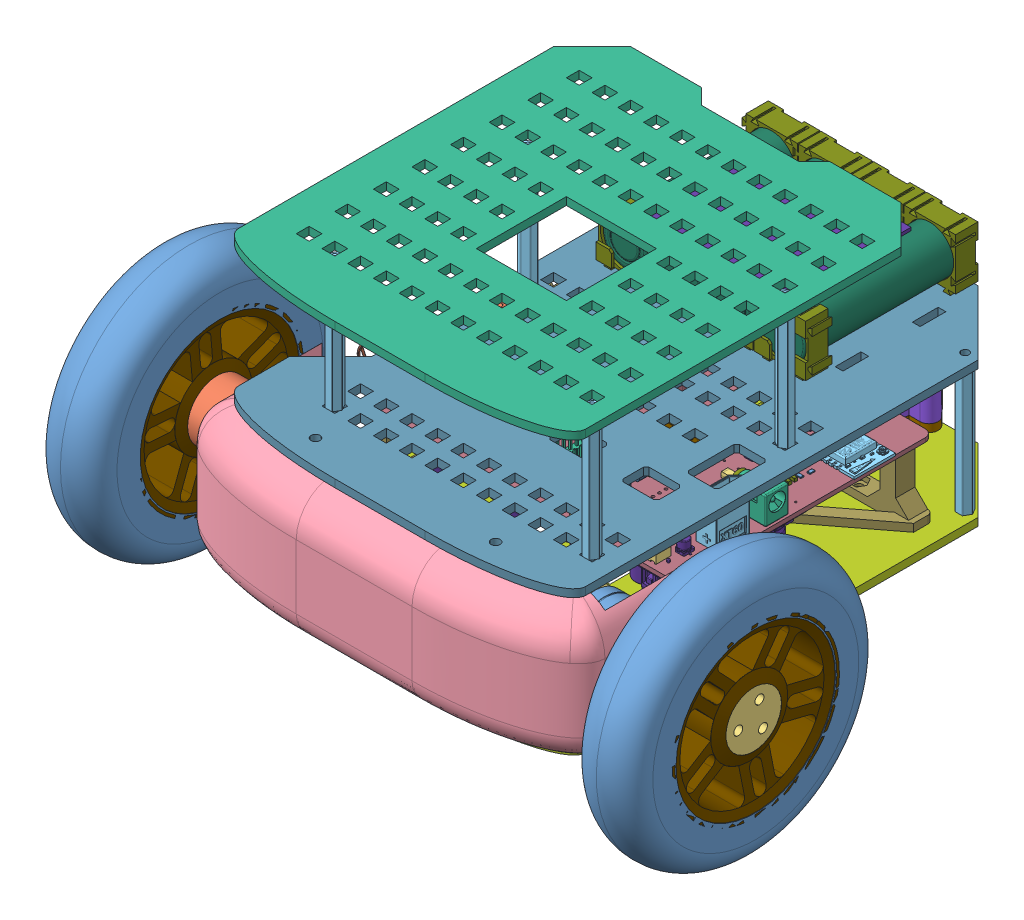
SolidWorks assembly main_assembly, configuration Predeterminado. Lengths in mm.
Overall size (232.39 147.84 245.63).
315 component instances, 64 part files, 45 mates.
Components (placement in the parent):
- JA25-371-12V-1: JA25-371-12V [Predeterminado] at (-23.0941 198.6621 54.477) x (0 0 1) z (-1 0 0) size (25 25 76.39)
  - Gearbox-1: Gearbox [Predeterminado] at (16.9623 5.2379 20.5646) size (25 25 21)
  - hub-1: hub [Predeterminado] at (16.9623 5.2379 39.5646) x (0.985611 -0.169031 0) z (0 0 1) size (6.95 6.95 4.5)
  - Motor-1: Motor [Predeterminado] at (16.9623 5.2379 -9.9354) size (24.2 24.2 30.5)
  - Axis-1: Axis [Predeterminado] at (16.9623 5.2379 39.5646) x (0.853161 0.521648 0) z (0 0 1) size (4 4 14)
  - PCB-1: PCB [Predeterminado] at (16.9623 5.2379 -11.4354) x (-1 0 0) z (0 0 -1) size (23 23 4.73)
  - Magnet-1: Magnet [Predeterminado] at (16.9623 5.2379 -17.3254) x (-0.17817 -0.984 0) z (0 0 -1) size (14.2 14.2 15.5)
- JA25-371-12V-2: JA25-371-12V [Predeterminado] at (42.7766 209.1379 54.477) x (0 0 1) z (1 0 0) size (25 25 76.39)
  - Gearbox-1: Gearbox [Predeterminado] at (16.9623 5.2379 20.5646) size (25 25 21)
  - hub-1: hub [Predeterminado] at (16.9623 5.2379 39.5646) x (0.985611 -0.169031 0) z (0 0 1) size (6.95 6.95 4.5)
  - Motor-1: Motor [Predeterminado] at (16.9623 5.2379 -9.9354) size (24.2 24.2 30.5)
  - Axis-1: Axis [Predeterminado] at (16.9623 5.2379 39.5646) x (0.853161 0.521648 0) z (0 0 1) size (4 4 14)
  - PCB-1: PCB [Predeterminado] at (16.9623 5.2379 -11.4354) x (-1 0 0) z (0 0 -1) size (23 23 4.73)
  - Magnet-1: Magnet [Predeterminado] at (16.9623 5.2379 -17.3254) x (-0.17817 -0.984 0) z (0 0 -1) size (14.2 14.2 15.5)
- base_noah-1: base_noah [Predeterminado] at (9.8412 177.5 6.4393) size (135.31 3.5 190.25)
- CasterJoint-1: CasterJoint [Default] at (-10.4939 224.3692 -36.408) x (1 0 0) z (0 0 -1) size (61 48.46 48.78)
  - C000-1: C000 [Default] at (20.3352 23.8692 48.4027) size (61 17 46)
  - C001-1: C001 [Default] at (20.3352 23.8692 48.4027) size (61 16.32 46)
  - BALL6MM-1: BALL6MM [Predeterminado] at (22.8352 26.8692 52.7329) size (6 6 6)
  - BALL40MM-1: BALL40MM [Default] at (20.3352 49.3191 48.4027) x (0.992761 -0.035378 0.11478) z (-0.109645 0.123176 0.986309) size (40 40 40)
  - BALL6MM-2: BALL6MM [Predeterminado] at (22.8352 26.8692 44.0726) size (6 6 6)
  - BALL6MM-3: BALL6MM [Predeterminado] at (15.3352 26.8692 48.4027) size (6 6 6)
  - pan head cross collar screw_din-1: pan head cross collar screw_din [DIN 967 - M3 x 10 - Z --- 9C] at (-6.6648 46.2192 48.6527) x (0 -1 0) z (0.01313 0 0.999914) size (12.25 7.5 7.5) (hidden)
  - pan head cross collar screw_din-2: pan head cross collar screw_din [DIN 967 - M3 x 10 - Z --- 9C] at (47.3352 46.2192 48.6527) x (0 -1 0) z (0 0 1) size (12.25 7.5 7.5) (hidden)
- pcb_holder_noah-1: pcb_holder_noah [Default] at (-2.6116 180.5 18.9157) x (-1 0 0) z (0 0 -1) size (120 28 100)
- power_button_noah-1: power_button_noah [Default] at (-42.6588 193.5 -36.0607) x (0 0 1) z (-1 0 0) size (25 20 7.5)
- noah_v02-1: noah_v02 [Default] at (159.8412 208.5 96.4393) x (-1 0 0) z (0 1 0) size (125.96 104.91 49.76)
  - noah_v02.step-1: noah_v02.step [Default] at origin size (125.96 104.91 49.76)
    - IDC-Header_2x05_P2.54mm_Vertical.step-1: IDC-Header_2x05_P2.54mm_Vertical.step [Default] at (176.6 -132.6 1.65) x (-0.707107 0.707107 0) z (0 0 1) size (9.1 20.36 12.1)
      - SOLID.step-1: SOLID.step [Default] at origin size (9.1 20.36 12.1)
    - DFN-8-1EP_3x3mm_P0.5mm_EP1.66x2.38mm.step-1: DFN-8-1EP_3x3mm_P0.5mm_EP1.66x2.38mm.step [Default] at (105.305 -107.385 1.65) x (0 1 0) z (0 0 1) size (3 2.98 0.77)
      - SOLID-0.step-1: SOLID-0.step [Default] at origin size (3 2.98 0.77)
    - C_0805_2012Metric.step-1: C_0805_2012Metric.step [Default] at (160.4 -70.1 1.65) x (0 -1 0) z (0 0 1) size (2 1.25 1.25)
      - SOLID-1.step-1: SOLID-1.step [Default] at origin size (2 1.25 1.25)
    - CP_Elec_4x4.5.step-1: CP_Elec_4x4.5.step [Default] at (140.6 -65.3 1.65) x (0 -1 0) z (0 0 1) size (5.74 5.46 4.5)
      - SOLID-2.step-1: SOLID-2.step [Default] at origin size (5.74 5.46 4.5)
    - C_0805_2012Metric.step-2: C_0805_2012Metric.step [Default] at (115.6 -134.6 1.65) size (2 1.25 1.25)
      - SOLID-1.step-1: SOLID-1.step [Default] at origin size (2 1.25 1.25)
    - CP_Elec_4x4.5.step-2: CP_Elec_4x4.5.step [Default] at (114.6 -129.4 1.65) x (0 1 0) z (0 0 1) size (5.74 5.46 4.5)
      - SOLID-2.step-1: SOLID-2.step [Default] at origin size (5.74 5.46 4.5)
    - PinSocket_1x06_P2.54mm_Vertical.step-1: PinSocket_1x06_P2.54mm_Vertical.step [Default] at (153.2 -146.2 1.65) x (0 -1 0) z (0 0 1) size (2.54 15.24 10.1)
      - SOLID-3.step-1: SOLID-3.step [Default] at origin size (2.54 15.24 10.1)
    - PinSocket_2x06_P2.54mm_Vertical.step-1: PinSocket_2x06_P2.54mm_Vertical.step [Default] at (153.2 -142.6 1.65) x (0 -1 0) z (0 0 1) size (5.08 15.24 10.1)
      - SOLID-4.step-1: SOLID-4.step [Default] at origin size (5.08 15.24 10.1)
    - ublox_NEO-6M.step-1: ublox_NEO-6M.step [Default] at (181.8 -59.6 11.65) x (0 1 0) z (1 0 0) size (39.06 22.61 48.01)
      - COMPOUND.step-1: COMPOUND.step [Default] at origin size (39.06 22.61 48.01)
    - D_SMA.step-1: D_SMA.step [Default] at (198.4 -143.2 1.65) x (-1 0 0) z (0 0 1) size (5 2.7 2.22)
      - SOLID-5.step-1: SOLID-5.step [Default] at origin size (5 2.7 2.22)
    - PinHeader_1x03_P2.54mm_Vertical.step-1: PinHeader_1x03_P2.54mm_Vertical.step [Default] at (105.6 -147.4 1.65) x (-1 0 0) z (0 0 1) size (2.54 7.62 11.54)
      - SOLID-6.step-1: SOLID-6.step [Default] at origin size (2.54 7.62 11.54)
    - C_0805_2012Metric.step-3: C_0805_2012Metric.step [Default] at (101.3 -107.1 1.65) x (-1 0 0) z (0 0 1) size (2 1.25 1.25)
      - SOLID-1.step-1: SOLID-1.step [Default] at origin size (2 1.25 1.25)
    - C_0805_2012Metric.step-4: C_0805_2012Metric.step [Default] at (101.3 -104.8 1.65) x (-1 0 0) z (0 0 1) size (2 1.25 1.25)
      - SOLID-1.step-1: SOLID-1.step [Default] at origin size (2 1.25 1.25)
    - ESP07.step-1: ESP07.step [Default] at (101.6 -127.3 1.65) x (0 1 0) z (1 0 0) size (19.34 14.61 27.24)
      - COMPOUND-7.step-1: COMPOUND-7.step [Default] at origin size (19.34 14.61 27.24)
    - Power_Barrel_Connector_Jack_694106301002.step-1: Power_Barrel_Connector_Jack_694106301002.step [Default] at (104.13 -90.01 1.65) x (0 -1 0) z (0 0 1) size (9.49 14.48 14.52)
      - COMPOUND-8.step-1: COMPOUND-8.step [Default] at origin size (9.49 14.48 14.52)
    - GY-91.step-1: GY-91.step [Default] at (119 -134.7 9.65) size (14.4 21 11.75)
      - COMPOUND-9.step-1: COMPOUND-9.step [Default] at origin size (14.4 21 11.75)
    - Tact_Switch_4.5mm_SMT.step-1: Tact_Switch_4.5mm_SMT.step [Default] at (139.14 -127.61 1.65) x (0 1 0) z (0 0 1) size (7.5 4.5 4.2)
      - COMPOUND-10.step-1: COMPOUND-10.step [Default] at origin size (7.5 4.5 4.2)
    - Tact_Switch_4.5mm_SMT.step-2: Tact_Switch_4.5mm_SMT.step [Default] at (167.3 -90.93 1.65) x (0 -1 0) z (0 0 1) size (7.5 4.5 4.2)
      - COMPOUND-10.step-1: COMPOUND-10.step [Default] at origin size (7.5 4.5 4.2)
    - tb5p-2p_p5_l10_w7-6_h10.step-1: tb5p-2p_p5_l10_w7-6_h10.step [Default] at (205.55 -62.68 6.65) x (0 1 0) z (1 0 0) size (10.6 14.1 7.6)
      - COMPOUND-11.step-1: COMPOUND-11.step [Default] at origin size (10.6 14.1 7.6)
    - SW_DIP_SPSTx02_Slide_6.7x6.64mm_W7.62mm_P2.54mm_LowProfile.step-1: SW_DIP_SPSTx02_Slide_6.7x6.64mm_W7.62mm_P2.54mm_LowProfile.step [Default] at (131.45 -139.55 1.65) x (-1 0 0) z (0 0 1) size (6.64 7.82 6)
      - SOLID-12.step-1: SOLID-12.step [Default] at origin size (6.64 7.82 6)
    - LQFP-100_14x14mm_P0.5mm.step-1: LQFP-100_14x14mm_P0.5mm.step [Default] at (161.4 -120.1 1.65) x (0.707107 -0.707107 0) z (0 0 1) size (16 16 1.5)
      - SOLID-13.step-1: SOLID-13.step [Default] at origin size (16 16 1.5)
    - USB_Mini-B_Lumberg_2486_01_Horizontal.step-1: USB_Mini-B_Lumberg_2486_01_Horizontal.step [Default] at (203.6 -123.9 1.65) x (0 1 0) z (0 0 1) size (9.9 9.21 5)
      - SOLID-14.step-1: SOLID-14.step [Default] at origin size (9.9 9.21 5)
    - Crystal_HC49-U_Vertical.step-1: Crystal_HC49-U_Vertical.step [Default] at (151.7 -106.6 1.65) x (-0.707107 -0.707107 0) z (0 0 1) size (10.9 4.65 16)
      - SOLID-15.step-1: SOLID-15.step [Default] at origin size (10.9 4.65 16)
    - SOIC-8_3.9x4.9mm_P1.27mm.step-1: SOIC-8_3.9x4.9mm_P1.27mm.step [Default] at (190.4 -107.7 1.65) size (6 4.9 1.75)
      - SOLID-16.step-1: SOLID-16.step [Default] at origin size (6 4.9 1.75)
    - SOT-23-5.step-1: SOT-23-5.step [Default] at (201.6 -138 1.65) size (2.8 2.9 1.55)
      - SOLID-17.step-1: SOLID-17.step [Default] at origin size (2.8 2.9 1.55)
    - SOT-23-6.step-1: SOT-23-6.step [Default] at (193.5 -124.3 1.65) size (2.8 2.9 1.55)
      - SOLID-18.step-1: SOLID-18.step [Default] at origin size (2.8 2.9 1.55)
    - XL4015_StepDown_DC-DC_5A_(CC-CV)_v1.step-1: XL4015_StepDown_DC-DC_5A_(CC-CV)_v1.step [Default] at (119.3 -102.3 -0.05) x (0 1 0) z (0 0 -1) size (51 26 18.15)
      - COMPOUND-19.step-1: COMPOUND-19.step [Default] at origin size (51 26 18.15)
    - XL4015_StepDown_DC-DC_5A_(CC-CV)_v1.step-2: XL4015_StepDown_DC-DC_5A_(CC-CV)_v1.step [Default] at (147.1 -102.4 -0.05) x (0 1 0) z (0 0 -1) size (51 26 18.15)
      - COMPOUND-19.step-1: COMPOUND-19.step [Default] at origin size (51 26 18.15)
    - XL4015_StepDown_DC-DC_5A_(CC-CV)_v1.step-3: XL4015_StepDown_DC-DC_5A_(CC-CV)_v1.step [Default] at (174.9 -102.3 -0.05) x (0 1 0) z (0 0 -1) size (51 26 18.15)
      - COMPOUND-19.step-1: COMPOUND-19.step [Default] at origin size (51 26 18.15)
    - XL4015_StepDown_DC-DC_5A_(CC-CV)_v1.step-4: XL4015_StepDown_DC-DC_5A_(CC-CV)_v1.step [Default] at (91.5 -102.3 -0.05) x (0 1 0) z (0 0 -1) size (51 26 18.15)
      - COMPOUND-19.step-1: COMPOUND-19.step [Default] at origin size (51 26 18.15)
    - TB6612FNG_Motor_Driver.step-1: TB6612FNG_Motor_Driver.step [Default] at (130.68 -80.59 11.65) x (0 0 1) z (1 0 0) size (3.57 20.98 20.9)
      - SOLID-20.step-1: SOLID-20.step [Default] at origin size (3.57 20.98 20.9)
    - R_0805_2012Metric.step-1: R_0805_2012Metric.step [Default] at (168.4 -107.4 1.65) x (0.707107 -0.707107 0) z (0 0 1) size (2 1.2 0.45)
      - SOLID-21.step-1: SOLID-21.step [Default] at origin size (2 1.2 0.45)
    - R_0805_2012Metric.step-2: R_0805_2012Metric.step [Default] at (200.7 -105.4 1.65) x (0 1 0) z (0 0 1) size (2 1.2 0.45)
      - SOLID-21.step-1: SOLID-21.step [Default] at origin size (2 1.2 0.45)
    - R_0805_2012Metric.step-3: R_0805_2012Metric.step [Default] at (200.7 -109.4 1.65) x (0 -1 0) z (0 0 1) size (2 1.2 0.45)
      - SOLID-21.step-1: SOLID-21.step [Default] at origin size (2 1.2 0.45)
    - R_0805_2012Metric.step-4: R_0805_2012Metric.step [Default] at (197.3 -105.4 1.65) x (0 1 0) z (0 0 1) size (2 1.2 0.45)
      - SOLID-21.step-1: SOLID-21.step [Default] at origin size (2 1.2 0.45)
    - R_0805_2012Metric.step-5: R_0805_2012Metric.step [Default] at (197.3 -109.4 1.65) x (0 -1 0) z (0 0 1) size (2 1.2 0.45)
      - SOLID-21.step-1: SOLID-21.step [Default] at origin size (2 1.2 0.45)
    - R_0805_2012Metric.step-6: R_0805_2012Metric.step [Default] at (192.1 -103.5 1.65) size (2 1.2 0.45)
      - SOLID-21.step-1: SOLID-21.step [Default] at origin size (2 1.2 0.45)
    - R_0805_2012Metric.step-7: R_0805_2012Metric.step [Default] at (201.6 -131.9 1.65) x (-1 0 0) z (0 0 1) size (2 1.2 0.45)
      - SOLID-21.step-1: SOLID-21.step [Default] at origin size (2 1.2 0.45)
    - R_0805_2012Metric.step-8: R_0805_2012Metric.step [Default] at (193.5 -120.9 1.65) size (2 1.2 0.45)
      - SOLID-21.step-1: SOLID-21.step [Default] at origin size (2 1.2 0.45)
    - R_0805_2012Metric.step-9: R_0805_2012Metric.step [Default] at (192.9 -127.5 1.65) x (-1 0 0) z (0 0 1) size (2 1.2 0.45)
      - SOLID-21.step-1: SOLID-21.step [Default] at origin size (2 1.2 0.45)
    - R_0805_2012Metric.step-10: R_0805_2012Metric.step [Default] at (192.9 -129.9 1.65) size (2 1.2 0.45)
      - SOLID-21.step-1: SOLID-21.step [Default] at origin size (2 1.2 0.45)
    - R_0805_2012Metric.step-11: R_0805_2012Metric.step [Default] at (110.6 -141.6 1.65) size (2 1.2 0.45)
      - SOLID-21.step-1: SOLID-21.step [Default] at origin size (2 1.2 0.45)
    - R_0805_2012Metric.step-12: R_0805_2012Metric.step [Default] at (177.2 -71.9 1.65) x (-1 0 0) z (0 0 1) size (2 1.2 0.45)
      - SOLID-21.step-1: SOLID-21.step [Default] at origin size (2 1.2 0.45)
    - R_0805_2012Metric.step-13: R_0805_2012Metric.step [Default] at (177.2 -65.3 1.65) x (-1 0 0) z (0 0 1) size (2 1.2 0.45)
      - SOLID-21.step-1: SOLID-21.step [Default] at origin size (2 1.2 0.45)
    - R_0805_2012Metric.step-14: R_0805_2012Metric.step [Default] at (177.2 -69.7 1.65) x (-1 0 0) z (0 0 1) size (2 1.2 0.45)
      - SOLID-21.step-1: SOLID-21.step [Default] at origin size (2 1.2 0.45)
    - R_0805_2012Metric.step-15: R_0805_2012Metric.step [Default] at (177.2 -67.5 1.65) x (-1 0 0) z (0 0 1) size (2 1.2 0.45)
      - SOLID-21.step-1: SOLID-21.step [Default] at origin size (2 1.2 0.45)
    - R_0805_2012Metric.step-16: R_0805_2012Metric.step [Default] at (165.3 -97.8 1.65) x (0 1 0) z (0 0 1) size (2 1.2 0.45)
      - SOLID-21.step-1: SOLID-21.step [Default] at origin size (2 1.2 0.45)
    - R_0805_2012Metric.step-17: R_0805_2012Metric.step [Default] at (152.4 -93.8 1.65) x (0 -1 0) z (0 0 1) size (2 1.2 0.45)
      - SOLID-21.step-1: SOLID-21.step [Default] at origin size (2 1.2 0.45)
    - R_0805_2012Metric.step-18: R_0805_2012Metric.step [Default] at (155.2 -93.8 1.65) x (0 -1 0) z (0 0 1) size (2 1.2 0.45)
      - SOLID-21.step-1: SOLID-21.step [Default] at origin size (2 1.2 0.45)
    - R_0805_2012Metric.step-19: R_0805_2012Metric.step [Default] at (192.9 -132.2 1.65) x (-1 0 0) z (0 0 1) size (2 1.2 0.45)
      - SOLID-21.step-1: SOLID-21.step [Default] at origin size (2 1.2 0.45)
    - R_0805_2012Metric.step-20: R_0805_2012Metric.step [Default] at (169 -104.8 1.65) x (0.707107 -0.707107 0) z (0 0 1) size (2 1.2 0.45)
      - SOLID-21.step-1: SOLID-21.step [Default] at origin size (2 1.2 0.45)
    - R_0805_2012Metric.step-21: R_0805_2012Metric.step [Default] at (174.7 -105.9 1.65) size (2 1.2 0.45)
      - SOLID-21.step-1: SOLID-21.step [Default] at origin size (2 1.2 0.45)
    - R_0805_2012Metric.step-22: R_0805_2012Metric.step [Default] at (111.4 -74.4 1.65) x (0 1 0) z (0 0 1) size (2 1.2 0.45)
      - SOLID-21.step-1: SOLID-21.step [Default] at origin size (2 1.2 0.45)
    - R_0805_2012Metric.step-23: R_0805_2012Metric.step [Default] at (110.4 -77.6 1.65) x (-1 0 0) z (0 0 1) size (2 1.2 0.45)
      - SOLID-21.step-1: SOLID-21.step [Default] at origin size (2 1.2 0.45)
    - R_0805_2012Metric.step-24: R_0805_2012Metric.step [Default] at (101.3 -109.5 1.65) size (2 1.2 0.45)
      - SOLID-21.step-1: SOLID-21.step [Default] at origin size (2 1.2 0.45)
    - R_0805_2012Metric.step-25: R_0805_2012Metric.step [Default] at (100.5 -113.1 1.65) x (0 -1 0) z (0 0 1) size (2 1.2 0.45)
      - SOLID-21.step-1: SOLID-21.step [Default] at origin size (2 1.2 0.45)
    - R_0805_2012Metric.step-26: R_0805_2012Metric.step [Default] at (115.4 -147.6 1.65) size (2 1.2 0.45)
      - SOLID-21.step-1: SOLID-21.step [Default] at origin size (2 1.2 0.45)
    - R_0805_2012Metric.step-27: R_0805_2012Metric.step [Default] at (115.4 -145.4 1.65) size (2 1.2 0.45)
      - SOLID-21.step-1: SOLID-21.step [Default] at origin size (2 1.2 0.45)
    - R_0805_2012Metric.step-28: R_0805_2012Metric.step [Default] at (115.4 -143.2 1.65) size (2 1.2 0.45)
      - SOLID-21.step-1: SOLID-21.step [Default] at origin size (2 1.2 0.45)
    - R_0805_2012Metric.step-29: R_0805_2012Metric.step [Default] at (115.4 -141 1.65) size (2 1.2 0.45)
      - SOLID-21.step-1: SOLID-21.step [Default] at origin size (2 1.2 0.45)
    - R_2512_6332Metric.step-1: R_2512_6332Metric.step [Default] at (105.2 -100.8 1.65) size (6.3 3.2 0.6)
      - SOLID-22.step-1: SOLID-22.step [Default] at origin size (6.3 3.2 0.6)
    - R_0805_2012Metric.step-30: R_0805_2012Metric.step [Default] at (104 -112.2 1.65) x (-1 0 0) z (0 0 1) size (2 1.2 0.45)
      - SOLID-21.step-1: SOLID-21.step [Default] at origin size (2 1.2 0.45)
    - R_0805_2012Metric.step-31: R_0805_2012Metric.step [Default] at (104 -114.4 1.65) x (-1 0 0) z (0 0 1) size (2 1.2 0.45)
      - SOLID-21.step-1: SOLID-21.step [Default] at origin size (2 1.2 0.45)
    - R_0805_2012Metric.step-32: R_0805_2012Metric.step [Default] at (118.1 -81.9 1.65) x (-1 0 0) z (0 0 1) size (2 1.2 0.45)
      - SOLID-21.step-1: SOLID-21.step [Default] at origin size (2 1.2 0.45)
    - Molex_KK-254_AE-6410-04A_1x04_P2.54mm_Vertical.step-1: Molex_KK-254_AE-6410-04A_1x04_P2.54mm_Vertical.step [Default] at (205.6 -95.2 1.65) x (0 -1 0) z (0 0 1) size (10.16 5.8 15.26)
      - SOLID-23.step-1: SOLID-23.step [Default] at origin size (10.16 5.8 15.26)
    - Molex_KK-254_AE-6410-06A_1x06_P2.54mm_Vertical.step-1: Molex_KK-254_AE-6410-06A_1x06_P2.54mm_Vertical.step [Default] at (192 -144.6 1.65) x (-1 0 0) z (0 0 1) size (15.24 5.8 15.26)
      - SOLID-24.step-1: SOLID-24.step [Default] at origin size (15.24 5.8 15.26)
    - Molex_KK-254_AE-6410-04A_1x04_P2.54mm_Vertical.step-2: Molex_KK-254_AE-6410-04A_1x04_P2.54mm_Vertical.step [Default] at (205.6 -70.8 1.65) x (0 -1 0) z (0 0 1) size (10.16 5.8 15.26)
      - SOLID-23.step-1: SOLID-23.step [Default] at origin size (10.16 5.8 15.26)
    - Molex_KK-254_AE-6410-04A_1x04_P2.54mm_Vertical.step-3: Molex_KK-254_AE-6410-04A_1x04_P2.54mm_Vertical.step [Default] at (205.6 -107.4 1.65) x (0 -1 0) z (0 0 1) size (10.16 5.8 15.26)
      - SOLID-23.step-1: SOLID-23.step [Default] at origin size (10.16 5.8 15.26)
    - Molex_KK-254_AE-6410-04A_1x04_P2.54mm_Vertical.step-4: Molex_KK-254_AE-6410-04A_1x04_P2.54mm_Vertical.step [Default] at (205.6 -83 1.65) x (0 -1 0) z (0 0 1) size (10.16 5.8 15.26)
      - SOLID-23.step-1: SOLID-23.step [Default] at origin size (10.16 5.8 15.26)
    - PinHeader_1x03_P2.54mm_Vertical.step-2: PinHeader_1x03_P2.54mm_Vertical.step [Default] at (163.25 -146.15 1.65) x (-1 0 0) z (0 0 1) size (2.54 7.62 11.54)
      - SOLID-6.step-1: SOLID-6.step [Default] at origin size (2.54 7.62 11.54)
    - PinHeader_1x03_P2.54mm_Vertical.step-3: PinHeader_1x03_P2.54mm_Vertical.step [Default] at (167.05 -146.15 1.65) x (-1 0 0) z (0 0 1) size (2.54 7.62 11.54)
      - SOLID-6.step-1: SOLID-6.step [Default] at origin size (2.54 7.62 11.54)
    - PinHeader_1x03_P2.54mm_Vertical.step-4: PinHeader_1x03_P2.54mm_Vertical.step [Default] at (170.85 -146.15 1.65) x (-1 0 0) z (0 0 1) size (2.54 7.62 11.54)
      - SOLID-6.step-1: SOLID-6.step [Default] at origin size (2.54 7.62 11.54)
    - PinHeader_1x03_P2.54mm_Vertical.step-5: PinHeader_1x03_P2.54mm_Vertical.step [Default] at (174.65 -146.15 1.65) x (-1 0 0) z (0 0 1) size (2.54 7.62 11.54)
      - SOLID-6.step-1: SOLID-6.step [Default] at origin size (2.54 7.62 11.54)
    - Molex_KK-254_AE-6410-04A_1x04_P2.54mm_Vertical.step-5: Molex_KK-254_AE-6410-04A_1x04_P2.54mm_Vertical.step [Default] at (108.5 -54.8 1.65) x (-1 0 0) z (0 0 1) size (10.16 5.8 15.26)
      - SOLID-23.step-1: SOLID-23.step [Default] at origin size (10.16 5.8 15.26)
    - Molex_KK-254_AE-6410-04A_1x04_P2.54mm_Vertical.step-6: Molex_KK-254_AE-6410-04A_1x04_P2.54mm_Vertical.step [Default] at (163.9 -55 1.65) x (-1 0 0) z (0 0 1) size (10.16 5.8 15.26)
      - SOLID-23.step-1: SOLID-23.step [Default] at origin size (10.16 5.8 15.26)
    - XT60_Male_Connector.step-1: XT60_Male_Connector.step [Default] at (95.7 -75.4 17.65) x (0 1 0) z (-1 0 0) size (15.93 20.03 8.13)
      - COMPOUND-25.step-1: COMPOUND-25.step [Default] at origin size (15.93 20.03 8.13)
    - Molex_KK-254_AE-6410-04A_1x04_P2.54mm_Vertical.step-7: Molex_KK-254_AE-6410-04A_1x04_P2.54mm_Vertical.step [Default] at (136.5 -54.8 1.65) x (-1 0 0) z (0 0 1) size (10.16 5.8 15.26)
      - SOLID-23.step-1: SOLID-23.step [Default] at origin size (10.16 5.8 15.26)
    - Molex_KK-254_AE-6410-04A_1x04_P2.54mm_Vertical.step-8: Molex_KK-254_AE-6410-04A_1x04_P2.54mm_Vertical.step [Default] at (191.5 -54.9 1.65) x (-1 0 0) z (0 0 1) size (10.16 5.8 15.26)
      - SOLID-23.step-1: SOLID-23.step [Default] at origin size (10.16 5.8 15.26)
    - PinHeader_1x06_P2.54mm_Vertical.step-1: PinHeader_1x06_P2.54mm_Vertical.step [Default] at (152.6 -76.7 1.65) x (-1 0 0) z (0 0 1) size (2.54 15.24 11.54)
      - SOLID-26.step-1: SOLID-26.step [Default] at origin size (2.54 15.24 11.54)
    - PinHeader_1x06_P2.54mm_Vertical.step-2: PinHeader_1x06_P2.54mm_Vertical.step [Default] at (145.8 -76.74 1.65) x (-1 0 0) z (0 0 1) size (2.54 15.24 11.54)
      - SOLID-26.step-1: SOLID-26.step [Default] at origin size (2.54 15.24 11.54)
    - C_Disc_D7.5mm_W2.5mm_P5.00mm.step-1: C_Disc_D7.5mm_W2.5mm_P5.00mm.step [Default] at (108 -95 1.65) x (0 1 0) z (0 0 1) size (7.5 2.5 9.6)
      - SOLID-27.step-1: SOLID-27.step [Default] at origin size (7.5 2.5 9.6)
    - LED_1206_3216Metric.step-1: LED_1206_3216Metric.step [Default] at (206.8 -131.9 1.65) x (-1 0 0) z (0 0 1) size (3.2 1.6 1.1)
      - SOLID-28.step-1: SOLID-28.step [Default] at origin size (3.2 1.6 1.1)
    - D_SMA.step-2: D_SMA.step [Default] at (197.2 -136 1.65) x (0 1 0) z (0 0 1) size (5 2.7 2.22)
      - SOLID-5.step-1: SOLID-5.step [Default] at origin size (5 2.7 2.22)
    - D_SOD-323.step-1: D_SOD-323.step [Default] at (119.9 -147.5 1.65) size (2.5 1.25 1.1)
      - SOLID-29.step-1: SOLID-29.step [Default] at origin size (2.5 1.25 1.1)
    - D_SMA.step-3: D_SMA.step [Default] at (113.8 -95 1.65) x (-1 0 0) z (0 0 1) size (5 2.7 2.22)
      - SOLID-5.step-1: SOLID-5.step [Default] at origin size (5 2.7 2.22)
    - D_SMA.step-4: D_SMA.step [Default] at (115.8 -75.4 1.65) x (0 1 0) z (0 0 1) size (5 2.7 2.22)
      - SOLID-5.step-1: SOLID-5.step [Default] at origin size (5 2.7 2.22)
    - D_SMA.step-5: D_SMA.step [Default] at (104 -79.9 1.65) x (0 1 0) z (0 0 1) size (5 2.7 2.22)
      - SOLID-5.step-1: SOLID-5.step [Default] at origin size (5 2.7 2.22)
    - LED_1206_3216Metric.step-2: LED_1206_3216Metric.step [Default] at (152.4 -89 1.65) x (0 -1 0) z (0 0 1) size (3.2 1.6 1.1)
      - SOLID-28.step-1: SOLID-28.step [Default] at origin size (3.2 1.6 1.1)
    - LED_1206_3216Metric.step-3: LED_1206_3216Metric.step [Default] at (155.2 -89 1.65) x (0 -1 0) z (0 0 1) size (3.2 1.6 1.1)
      - SOLID-28.step-1: SOLID-28.step [Default] at origin size (3.2 1.6 1.1)
    - LED_1206_3216Metric.step-4: LED_1206_3216Metric.step [Default] at (192.4 -134.7 1.65) size (3.2 1.6 1.1)
      - SOLID-28.step-1: SOLID-28.step [Default] at origin size (3.2 1.6 1.1)
    - D_SOD-323.step-2: D_SOD-323.step [Default] at (110.7 -145.4 1.65) size (2.5 1.25 1.1)
      - SOLID-29.step-1: SOLID-29.step [Default] at origin size (2.5 1.25 1.1)
    - D_SOD-323.step-3: D_SOD-323.step [Default] at (119.9 -143.2 1.65) size (2.5 1.25 1.1)
      - SOLID-29.step-1: SOLID-29.step [Default] at origin size (2.5 1.25 1.1)
    - D_DO-41_SOD81_P10.16mm_Horizontal.step-1: D_DO-41_SOD81_P10.16mm_Horizontal.step [Default] at (131 -83.2 1.65) x (0 1 0) z (0 0 1) size (10.96 2.72 5.71)
      - SOLID-30.step-1: SOLID-30.step [Default] at origin size (10.96 2.72 5.71)
    - D_DO-41_SOD81_P10.16mm_Horizontal.step-2: D_DO-41_SOD81_P10.16mm_Horizontal.step [Default] at (136.1 -67.3 1.65) x (-1 0 0) z (0 0 1) size (10.96 2.72 5.71)
      - SOLID-30.step-1: SOLID-30.step [Default] at origin size (10.96 2.72 5.71)
    - D_DO-41_SOD81_P10.16mm_Horizontal.step-3: D_DO-41_SOD81_P10.16mm_Horizontal.step [Default] at (136.1 -63.7 1.65) x (-1 0 0) z (0 0 1) size (10.96 2.72 5.71)
      - SOLID-30.step-1: SOLID-30.step [Default] at origin size (10.96 2.72 5.71)
    - C_0805_2012Metric.step-5: C_0805_2012Metric.step [Default] at (160.8 -135.8 1.65) x (-0.707107 -0.707107 0) z (0 0 1) size (2 1.25 1.25)
      - SOLID-1.step-1: SOLID-1.step [Default] at origin size (2 1.25 1.25)
    - C_0603_1608Metric.step-1: C_0603_1608Metric.step [Default] at (193.96 -113.92 1.65) x (-1 0 0) z (0 0 1) size (1.6 0.8 0.8)
      - SOLID-31.step-1: SOLID-31.step [Default] at origin size (1.6 0.8 0.8)
    - C_0603_1608Metric.step-2: C_0603_1608Metric.step [Default] at (194 -112.2 1.65) x (-1 0 0) z (0 0 1) size (1.6 0.8 0.8)
      - SOLID-31.step-1: SOLID-31.step [Default] at origin size (1.6 0.8 0.8)
    - C_1206_3216Metric.step-1: C_1206_3216Metric.step [Default] at (206.8 -137.1 1.65) size (3.2 1.6 1.6)
      - SOLID-32.step-1: SOLID-32.step [Default] at origin size (3.2 1.6 1.6)
    - C_1206_3216Metric.step-2: C_1206_3216Metric.step [Default] at (206.8 -141.1 1.65) size (3.2 1.6 1.6)
      - SOLID-32.step-1: SOLID-32.step [Default] at origin size (3.2 1.6 1.6)
    - CP_Elec_4x4.5.step-3: CP_Elec_4x4.5.step [Default] at (116.6 -107.2 1.65) size (5.74 5.46 4.5)
      - SOLID-2.step-1: SOLID-2.step [Default] at origin size (5.74 5.46 4.5)
    - CP_Elec_4x4.5.step-4: CP_Elec_4x4.5.step [Default] at (98.8 -62 1.65) x (-1 0 0) z (0 0 1) size (5.74 5.46 4.5)
      - SOLID-2.step-1: SOLID-2.step [Default] at origin size (5.74 5.46 4.5)
    - C_0805_2012Metric.step-6: C_0805_2012Metric.step [Default] at (110.3 -84.1 1.65) size (2 1.25 1.25)
      - SOLID-1.step-1: SOLID-1.step [Default] at origin size (2 1.25 1.25)
    - CP_Elec_4x4.5.step-5: CP_Elec_4x4.5.step [Default] at (117.6 -60.5 1.65) x (-1 0 0) z (0 0 1) size (5.74 5.46 4.5)
      - SOLID-2.step-1: SOLID-2.step [Default] at origin size (5.74 5.46 4.5)
    - C_0805_2012Metric.step-7: C_0805_2012Metric.step [Default] at (168.1 -97.8 1.65) x (0 1 0) z (0 0 1) size (2 1.25 1.25)
      - SOLID-1.step-1: SOLID-1.step [Default] at origin size (2 1.25 1.25)
    - C_1206_3216Metric.step-3: C_1206_3216Metric.step [Default] at (176.8 -118 1.65) x (0.707107 0.707107 0) z (0 0 1) size (3.2 1.6 1.6)
      - SOLID-32.step-1: SOLID-32.step [Default] at origin size (3.2 1.6 1.6)
    - C_1206_3216Metric.step-4: C_1206_3216Metric.step [Default] at (178.6 -119.9 1.65) x (0.707107 0.707107 0) z (0 0 1) size (3.2 1.6 1.6)
      - SOLID-32.step-1: SOLID-32.step [Default] at origin size (3.2 1.6 1.6)
    - C_1206_3216Metric.step-5: C_1206_3216Metric.step [Default] at (157.3 -133.1 1.65) x (-0.707107 -0.707107 0) z (0 0 1) size (3.2 1.6 1.6)
      - SOLID-32.step-1: SOLID-32.step [Default] at origin size (3.2 1.6 1.6)
    - C_0603_1608Metric.step-3: C_0603_1608Metric.step [Default] at (145.2 -114.4 1.65) x (0.707107 -0.707107 0) z (0 0 1) size (1.6 0.8 0.8)
      - SOLID-31.step-1: SOLID-31.step [Default] at origin size (1.6 0.8 0.8)
    - C_0603_1608Metric.step-4: C_0603_1608Metric.step [Default] at (156.1 -103.5 1.65) x (0.707107 -0.707107 0) z (0 0 1) size (1.6 0.8 0.8)
      - SOLID-31.step-1: SOLID-31.step [Default] at origin size (1.6 0.8 0.8)
    - C_0805_2012Metric.step-8: C_0805_2012Metric.step [Default] at (150.6 -113.5 1.65) x (-0.707107 -0.707107 0) z (0 0 1) size (2 1.25 1.25)
      - SOLID-1.step-1: SOLID-1.step [Default] at origin size (2 1.25 1.25)
    - C_0805_2012Metric.step-9: C_0805_2012Metric.step [Default] at (147.7 -116.4 1.65) x (0.707107 0.707107 0) z (0 0 1) size (2 1.25 1.25)
      - SOLID-1.step-1: SOLID-1.step [Default] at origin size (2 1.25 1.25)
    - C_0805_2012Metric.step-10: C_0805_2012Metric.step [Default] at (156.6 -108.9 1.65) x (-0.707107 -0.707107 0) z (0 0 1) size (2 1.25 1.25)
      - SOLID-1.step-1: SOLID-1.step [Default] at origin size (2 1.25 1.25)
    - C_1206_3216Metric.step-6: C_1206_3216Metric.step [Default] at (146.9 -123.1 1.65) x (-0.707107 -0.707107 0) z (0 0 1) size (3.2 1.6 1.6)
      - SOLID-32.step-1: SOLID-32.step [Default] at origin size (3.2 1.6 1.6)
    - C_0805_2012Metric.step-11: C_0805_2012Metric.step [Default] at (166 -103.2 1.65) x (0.707107 0.707107 0) z (0 0 1) size (2 1.25 1.25)
      - SOLID-1.step-1: SOLID-1.step [Default] at origin size (2 1.25 1.25)
    - C_0805_2012Metric.step-12: C_0805_2012Metric.step [Default] at (148.9 -124.3 1.65) x (0.707107 0.707107 0) z (0 0 1) size (2 1.25 1.25)
      - SOLID-1.step-1: SOLID-1.step [Default] at origin size (2 1.25 1.25)
    - C_0805_2012Metric.step-13: C_0805_2012Metric.step [Default] at (159.2 -134.3 1.65) x (0.707107 0.707107 0) z (0 0 1) size (2 1.25 1.25)
      - SOLID-1.step-1: SOLID-1.step [Default] at origin size (2 1.25 1.25)
    - C_0805_2012Metric.step-14: C_0805_2012Metric.step [Default] at (174.8 -116.6 1.65) x (-0.707107 -0.707107 0) z (0 0 1) size (2 1.25 1.25)
      - SOLID-1.step-1: SOLID-1.step [Default] at origin size (2 1.25 1.25)
    - CP_Elec_4x4.5.step-6: CP_Elec_4x4.5.step [Default] at (117.6 -66.1 1.65) x (-1 0 0) z (0 0 1) size (5.74 5.46 4.5)
      - SOLID-2.step-1: SOLID-2.step [Default] at origin size (5.74 5.46 4.5)
    - COMPOUND-33.step-1: COMPOUND-33.step [Default] at origin size (120 100 1.6)
- top_noah-1: top_noah [Predeterminado] at (9.8412 230.5 6.4393) size (135.31 3.5 190.25)
- BatteryPack-1: BatteryPack [Predeterminado] at (20.658 196.5568 -100.8517) x (-1 0 0) z (0 1 0) size (86.68 67 25.44)
  - ELEB05-1: ELEB05 [По умолчанию] at (39.8212 13.291 48.4432) x (0.682904 0 -0.730508) z (0.730508 0 0.682904) size (18 65 18)
  - ELEB04-1: ELEB04 [Predeterminado] at (19.3212 20.991 48.4432) x (-1 0 0) z (0 0 1) size (21.5 8.7 21.5)
  - ELEB05-2: ELEB05 [По умолчанию] at (-1.1788 13.291 48.4432) x (0.778658 0 -0.627449) z (0.627449 0 0.778658) size (18 65 18)
  - ELEB05-3: ELEB05 [По умолчанию] at (-21.6788 78.291 48.4432) x (-0.837169 0 -0.546944) z (-0.546944 0 0.837169) size (18 65 18)
  - ELEB05-4: ELEB05 [По умолчанию] at (19.3212 78.291 48.4432) x (0.951676 0 -0.307103) z (-0.307103 0 -0.951676) size (18 65 18)
  - ELEB04-2: ELEB04 [Predeterminado] at (39.8212 70.591 48.4432) size (21.5 8.7 21.5)
  - ELEB04-3: ELEB04 [Predeterminado] at (-1.1788 70.591 48.4432) size (21.5 8.7 21.5)
  - ELEB04-4: ELEB04 [Predeterminado] at (19.3212 70.591 48.4432) size (21.5 8.7 21.5)
  - ELEB04-5: ELEB04 [Predeterminado] at (-21.6788 70.591 48.4432) size (21.5 8.7 21.5)
  - ELEB04-6: ELEB04 [Predeterminado] at (39.8212 20.991 48.4432) x (-1 0 0) z (0 0 1) size (21.5 8.7 21.5)
  - ELEB04-7: ELEB04 [Predeterminado] at (-21.6788 20.991 48.4432) x (-1 0 0) z (0 0 1) size (21.5 8.7 21.5)
  - ELEB04-8: ELEB04 [Predeterminado] at (-1.1788 20.991 48.4432) x (-1 0 0) z (0 0 1) size (21.5 8.7 21.5)
  - BMS-1: BMS [Default] at (8.3212 53.291 59.6432) x (-1 0 0) z (0 -1 0) size (60 1.2 50)
- TuxsWheel100mm-1: TuxsWheel100mm [Default] at (-171.2257 250.4557 113.3197) x (0 -0.988748 0.149588) z (1 0 0) size (114.18 114.18 36.69)
  - B02-1: B02 [Default] at (39.7671 48.3733 64.9228) size (90.04 90.04 24)
  - B021-1: B021 [Default] at (39.7671 48.3733 64.9228) x (0.988174 0.153337 0) z (0 0 1) size (100.02 100.02 24.11)
  - Adapter1-1: Adapter1 [Default] at (39.7671 48.3733 72.3069) x (0 -1 0) z (0 0 1) size (23 23 29.26)
  - Adapter2-1: Adapter2 [Default] at (39.7671 48.3733 65.8069) x (0 -1 0) z (0 0 1) size (21.7 21.7 6.5)
  - countersunk flat head cross recess screw_din-6: countersunk flat head cross recess screw_din [DIN EN ISO 7046-1 - M3 x 10 - Z - 10C] at (51.0178 48.3733 97.0669) x (-1 0 0) z (0 -0.928088 -0.37236) size (10 5.5 5.5) (hidden)
  - countersunk flat head cross recess screw_din-7: countersunk flat head cross recess screw_din [DIN EN ISO 7046-1 - M3 x 10 - Z - 10C] at (28.4595 48.3733 97.0669) x (1 0 0) z (0 0.306192 0.95197) size (10 5.5 5.5) (hidden)
  - countersunk flat head cross recess screw_din-8: countersunk flat head cross recess screw_din [DIN EN ISO 7046-1 - M3 x 10 - Z - 10C] at (36.7671 53.5694 65.4069) x (0 0 1) z (-0.331366 0.943502 0) size (10 5.5 5.5) (hidden)
  - countersunk flat head cross recess screw_din-9: countersunk flat head cross recess screw_din [DIN EN ISO 7046-1 - M3 x 10 - Z - 10C] at (36.7671 43.1771 65.4069) x (0 0 1) z (-0.394756 0.918786 0) size (10 5.5 5.5) (hidden)
  - countersunk flat head cross recess screw_din-10: countersunk flat head cross recess screw_din [DIN EN ISO 7046-1 - M3 x 10 - Z - 10C] at (45.7671 48.3733 65.4069) x (0 0 1) z (0.637808 -0.770196 0) size (10 5.5 5.5) (hidden)
  - hex thin nut gradeb_din-1: hex thin nut gradeb_din [Hexagon Nut ISO 4036 - M3 - C] at (33.3451 48.3733 97.0669) x (0 -1 0) z (-1 0 0) size (5.5 6.35 1.8) (hidden)
  - hex thin nut gradeb_din-2: hex thin nut gradeb_din [Hexagon Nut ISO 4036 - M3 - C] at (44.1892 48.3733 97.0669) x (0 -1 0) z (-1 0 0) size (5.5 6.35 1.8) (hidden)
- TuxsWheel100mm-2: TuxsWheel100mm [Default] at (190.9082 161.173 25.6594) x (0 -0.131432 0.991325) z (-1 0 0) size (114.18 114.18 36.69)
  - B02-1: B02 [Default] at (39.7671 48.3733 64.9228) size (90.04 90.04 24)
  - B021-1: B021 [Default] at (39.7671 48.3733 64.9228) x (0.988174 0.153337 0) z (0 0 1) size (100.02 100.02 24.11)
  - Adapter1-1: Adapter1 [Default] at (39.7671 48.3733 72.3069) x (0 -1 0) z (0 0 1) size (23 23 29.26)
  - Adapter2-1: Adapter2 [Default] at (39.7671 48.3733 65.8069) x (0 -1 0) z (0 0 1) size (21.7 21.7 6.5)
  - countersunk flat head cross recess screw_din-6: countersunk flat head cross recess screw_din [DIN EN ISO 7046-1 - M3 x 10 - Z - 10C] at (51.0178 48.3733 97.0669) x (-1 0 0) z (0 -0.928088 -0.37236) size (10 5.5 5.5) (hidden)
  - countersunk flat head cross recess screw_din-7: countersunk flat head cross recess screw_din [DIN EN ISO 7046-1 - M3 x 10 - Z - 10C] at (28.4595 48.3733 97.0669) x (1 0 0) z (0 0.306192 0.95197) size (10 5.5 5.5) (hidden)
  - countersunk flat head cross recess screw_din-8: countersunk flat head cross recess screw_din [DIN EN ISO 7046-1 - M3 x 10 - Z - 10C] at (36.7671 53.5694 65.4069) x (0 0 1) z (-0.331366 0.943502 0) size (10 5.5 5.5) (hidden)
  - countersunk flat head cross recess screw_din-9: countersunk flat head cross recess screw_din [DIN EN ISO 7046-1 - M3 x 10 - Z - 10C] at (36.7671 43.1771 65.4069) x (0 0 1) z (-0.394756 0.918786 0) size (10 5.5 5.5) (hidden)
  - countersunk flat head cross recess screw_din-10: countersunk flat head cross recess screw_din [DIN EN ISO 7046-1 - M3 x 10 - Z - 10C] at (45.7671 48.3733 65.4069) x (0 0 1) z (0.637808 -0.770196 0) size (10 5.5 5.5) (hidden)
  - hex thin nut gradeb_din-1: hex thin nut gradeb_din [Hexagon Nut ISO 4036 - M3 - C] at (33.3451 48.3733 97.0669) x (0 -1 0) z (-1 0 0) size (5.5 6.35 1.8) (hidden)
  - hex thin nut gradeb_din-2: hex thin nut gradeb_din [Hexagon Nut ISO 4036 - M3 - C] at (44.1892 48.3733 97.0669) x (0 -1 0) z (-1 0 0) size (5.5 6.35 1.8) (hidden)
- raspberryPi3B-1: raspberryPi3B [Detailed] at (12.5563 243.5 36.8223) x (0 0 -1) z (0 1 0) size (87.05 58.5 19.05) (hidden)
- front_noah-1: front_noah [Predeterminado] at (9.8412 180.5 81.4393) size (155.37 50.11 66.16)
- Spacer50mm_metal-1: Spacer50mm_metal [Varsayılan] at (-36.6588 230.5 -76.5607) x (-1 0 0) z (0 0 1) size (5.71 56.2 5)
- Spacer50mm_metal-2: Spacer50mm_metal [Varsayılan] at (72.3412 230.5 -63.5607) x (-1 0 0) z (0 0 1) size (5.71 56.2 5)
- Spacer50mm_metal-3: Spacer50mm_metal [Varsayılan] at (-32.1588 283.5 1.9393) x (-0.866025 0 -0.5) z (-0.5 0 0.866025) size (5.71 56.2 5)
- Spacer50mm_metal-4: Spacer50mm_metal [Varsayılan] at (67.8412 283.5 1.9393) x (-0.866025 0 0.5) z (0.5 0 0.866025) size (5.71 56.2 5)
- Spacer50mm_metal-5: Spacer50mm_metal [Varsayılan] at (67.8412 283.5 76.9393) x (-1 0 0) z (0 0 1) size (5.71 56.2 5)
- Spacer50mm_metal-6: Spacer50mm_metal [Varsayılan] at (-32.1588 283.5 76.9393) x (-1 0 0) z (0 0 1) size (5.71 56.2 5)
- shelf_noah-2: shelf_noah [Default] at (9.8412 283.5 26.4393) size (135.31 3.5 150.25)
Mates (geometry in assembly coordinates):
- Coincident127: coincident anti-aligned: plane of noah-1 through (9.8412 180.5 6.4393) normal (0 1 0); plane of CasterJoint-1/C001-1 through (36.8412 180.5 -85.0607) normal (0 -1 0)
- Concentric61: concentric aligned: cylinder of noah-1 through (36.8412 177.25 -85.0607) axis (0 1 0) radius 1.75; cylinder of CasterJoint-1/C000-1 through (36.8412 180.5 -85.0607) axis (0 1 0) radius 1.5
- Concentric62: concentric aligned: cylinder of noah-1 through (-17.1588 177.25 -85.0607) axis (0 1 0) radius 1.75; cylinder of CasterJoint-1/C000-1 through (-17.1588 180.5 -85.0607) axis (0 1 0) radius 1.5
- Concentric65: concentric anti-aligned: cylinder of noah-1 through (-46.4088 177.25 21.4393) axis (0 1 0) radius 1.75; cylinder of pcb_holder_noah-1 through (-46.4088 191.5 21.4393) axis (0 -1 0) radius 1.5
- Coincident130: coincident anti-aligned: plane of noah-1 through (9.8412 180.5 6.4393) normal (0 1 0); plane of pcb_holder_noah-1 through (-48.1588 180.5 44.4393) normal (0 -1 0)
- Concentric66: concentric anti-aligned: cylinder of noah-1 through (44.8412 177.25 -49.8107) axis (0 1 0) radius 1.75; cylinder of pcb_holder_noah-1 through (44.8412 191.5 -49.8107) axis (0 -1 0) radius 1.5
- Concentric67: concentric aligned: cylinder of pcb_holder_noah-1 through (-46.4088 193.5 -43.5607) axis (0 0 -1) radius 1.4933; cylinder of PowerButton-1 through (-46.4088 193.5 -26.0597) axis (0 0 -1) radius 1.5
- Coincident131: coincident anti-aligned: plane of pcb_holder_noah-1 through (-48.1588 183.5 44.4393) normal (0 1 0); plane of PowerButton-1 through (-50.1588 183.5 -46.0607) normal (0 -1 0)
- Coincident132: coincident anti-aligned: plane of pcb_holder_noah-1 through (69.8412 183.5 -46.0607) normal (0 0 1); plane of PowerButton-1 through (-50.1588 203.5 -46.0607) normal (0 0 -1)
- Coincident133: coincident anti-aligned: plane of pcb_holder_noah-1 through (-48.1588 208.5 -51.5607) normal (0 1 0); plane of noah_v02-1/noah_v02.step-1/COMPOUND-33.step-1 through (9.7787 208.5 -3.5084) normal (0 -1 0)
- Concentric68: concentric anti-aligned: circle of pcb_holder_noah-1; cylinder of noah_v02-1/noah_v02.step-1/COMPOUND-33.step-1 through (-48.1588 208.5 -51.5607) axis (0 -1 0) radius 2
- Coincident135: coincident aligned: plane of pcb_holder_noah-1 through (-50.1588 183.5 43.4393) normal (-1 0 0); plane of noah_v02-1/noah_v02.step-1/COMPOUND-33.step-1 through (-50.1588 208.5 -51.5607) normal (-1 0 0)
- Coincident154: coincident aligned: plane of top_noah-1 through (-57.6588 233.5 -88.5607) normal (0 0 -1); plane of BatteryPack-1/ELEB04-8 through (21.8367 245 -88.5607) normal (0 0 -1)
- Coincident155: coincident anti-aligned: plane of top_noah-1 through (9.8412 233.5 6.4393) normal (0 1 0); plane of BatteryPack-1/ELEB04-1 through (-3.7133 233.5 -79.8607) normal (0 -1 0)
- Concentric74: concentric anti-aligned: cylinder of JA25-371-12V-1/Axis-1 through (-76.6588 203.9 71.4393) axis (1 0 0) radius 2; cylinder of TuxsWheel100mm-1/Adapter1-1 through (-89.6588 203.9 71.4393) axis (-1 0 0) radius 2.1
- Concentric75: concentric anti-aligned: cylinder of JA25-371-12V-2/Axis-1 through (96.3412 203.9 71.4393) axis (-1 0 0) radius 2; cylinder of TuxsWheel100mm-2/Adapter1-1 through (109.3412 203.9 71.4393) axis (1 0 0) radius 2.1
- Parallel4: parallel anti-aligned: plane of BatteryPack-1/ELEB04-3 through (21.8367 245 -21.5607) normal (0 0 1); plane of raspberryPi3B-1 through (22.3063 258.1 -7.6777) normal (0 0 -1)
- Concentric76: concentric anti-aligned: cylinder of noah-1 through (59.8412 177.5 91.4393) axis (0 1 0) radius 1.75; cylinder of front_noah-1 through (59.8412 190.5 91.4393) axis (0 -1 0) radius 1.5
- Concentric77: concentric anti-aligned: cylinder of noah-1 through (37.3412 177.5 56.4393) axis (0 1 0) radius 1.75; cylinder of front_noah-1 through (37.3412 190.5 56.4393) axis (0 -1 0) radius 1.5
- Coincident156: coincident anti-aligned: plane of noah-1 through (9.8412 180.5 6.4393) normal (0 1 0); plane of front_noah-1 through (9.8412 180.5 81.4393) normal (0 -1 0)
- Coincident157: coincident anti-aligned: plane of JA25-371-12V-2/Gearbox-1 through (84.3412 203.9 71.4393) normal (1 0 0); plane of front_noah-1 through (84.3412 203.9 71.4393) normal (-1 0 0)
- Concentric78: concentric aligned: cylinder of JA25-371-12V-2/hub-1 through (86.8412 203.9 71.4393) axis (-1 0 0) radius 3.475; cylinder of front_noah-1 through (87.6162 203.9 71.4393) axis (-1 0 0) radius 3.75
- Concentric79: concentric anti-aligned: cylinder of JA25-371-12V-2/Gearbox-1 through (63.3412 203.9 80.1893) axis (1 0 0) radius 1.5; cylinder of front_noah-1 through (87.6162 203.9 80.1893) axis (-1 0 0) radius 1.75
- Concentric80: concentric aligned: cylinder of top_noah-1 through (44.8412 223.5 91.4393) axis (0 1 0) radius 1.75; cylinder of front_noah-1 through (44.8412 220.5 91.4393) axis (0 1 0) radius 1.5
- Coincident158: coincident anti-aligned: plane of JA25-371-12V-1/Gearbox-1 through (-64.6588 203.9 71.4393) normal (-1 0 0); plane of front_noah-1 through (-64.6588 31.3357 51.4393) normal (1 0 0)
- Concentric81: concentric anti-aligned: cylinder of JA25-371-12V-1/Axis-1 through (-76.6588 203.9 71.4393) axis (1 0 0) radius 2; cylinder of front_noah-1 through (87.6162 203.9 71.4393) axis (-1 0 0) radius 3.75
- Concentric82: concentric aligned: cylinder of JA25-371-12V-1/Gearbox-1 through (-43.6588 203.9 62.6893) axis (-1 0 0) radius 1.5; cylinder of front_noah-1 through (87.6162 203.9 62.6893) axis (-1 0 0) radius 1.75
- Distance1: distance = 2 mm anti-aligned: plane of TuxsWheel100mm-1/Adapter1-1 through (-69.6588 203.9 71.4393) normal (1 0 0); plane of front_noah-1 through (-67.6588 230.5 51.4393) normal (-1 0 0)
- Distance2: distance = 2 mm anti-aligned: plane of front_noah-1 through (87.3412 230.5 51.4393) normal (1 0 0); plane of TuxsWheel100mm-2/Adapter1-1 through (89.3412 203.9 71.4393) normal (-1 0 0)
- Concentric83: concentric aligned: cylinder of base_noah-1 through (-36.6588 177.25 -76.5607) axis (0 1 0) radius 1.75; cylinder of Spacer50mm_metal-1 through (-36.6588 179.3 -76.5607) axis (0 1 0) radius 1.3375
- Coincident159: coincident anti-aligned: plane of base_noah-1 through (9.8412 180.5 6.4393) normal (0 1 0); plane of Spacer50mm_metal-1 through (-36.6588 180.5 -76.5607) normal (0 -1 0)
- Coincident160: coincident anti-aligned: plane of base_noah-1 through (9.8412 180.5 6.4393) normal (0 1 0); plane of Spacer50mm_metal-2 through (72.3412 180.5 -63.5607) normal (0 -1 0)
- Concentric85: concentric aligned: cylinder of base_noah-1 through (72.3412 177.25 -63.5607) axis (0 1 0) radius 1.75; cylinder of Spacer50mm_metal-2 through (72.3412 179.3 -63.5607) axis (0 1 0) radius 1.3375
- Coincident162: coincident: point of top_noah-1; unknown of Spacer50mm_metal-6
- Coincident163: coincident anti-aligned: plane of top_noah-1 through (9.8412 233.5 6.4393) normal (0 1 0); plane of Spacer50mm_metal-5 through (67.8412 233.5 76.9393) normal (0 -1 0)
- Coincident165: coincident: unknown of top_noah-1; unknown of Spacer50mm_metal-5
- Coincident166: coincident: unknown of top_noah-1; unknown of Spacer50mm_metal-4
- Coincident167: coincident anti-aligned: plane of top_noah-1 through (9.8412 233.5 6.4393) normal (0 1 0); plane of Spacer50mm_metal-4 through (67.8412 233.5 1.9393) normal (0 -1 0)
- Coincident168: coincident anti-aligned: line of top_noah-1 through (70.3412 233.5 4.4393) axis (0 0 -1); line of Spacer50mm_metal-4 through (70.3412 233.5 0.6114) axis (0 0 1)
- Coincident169: coincident: unknown of top_noah-1; unknown of Spacer50mm_metal-3
- Coincident170: coincident: line of top_noah-1 through (-34.6588 233.5 -0.5607) axis (0 0 1); plane of Spacer50mm_metal-3 through (-34.6588 233.5 3.3827) normal (-1 0 0)
- Coincident171: coincident anti-aligned: plane of top_noah-1 through (9.8412 233.5 6.4393) normal (0 1 0); plane of Spacer50mm_metal-3 through (-32.1588 233.5 1.9393) normal (0 -1 0)
- Coincident172: coincident anti-aligned: plane of Spacer50mm_metal-4 through (67.8412 283.5 1.9393) normal (0 1 0); plane of shelf_noah-2 through (9.8412 283.5 26.4393) normal (0 -1 0)
- Coincident173: coincident aligned: plane of top_noah-1 through (77.3412 233.5 -88.5607) normal (1 0 0); plane of shelf_noah-2 through (77.3412 286.5 -48.5607) normal (1 0 0)
- Coincident174: coincident aligned: plane of top_noah-1 through (-57.6588 233.5 101.4393) normal (0 0 1); plane of shelf_noah-2 through (-57.6588 286.5 101.4393) normal (0 0 1)
